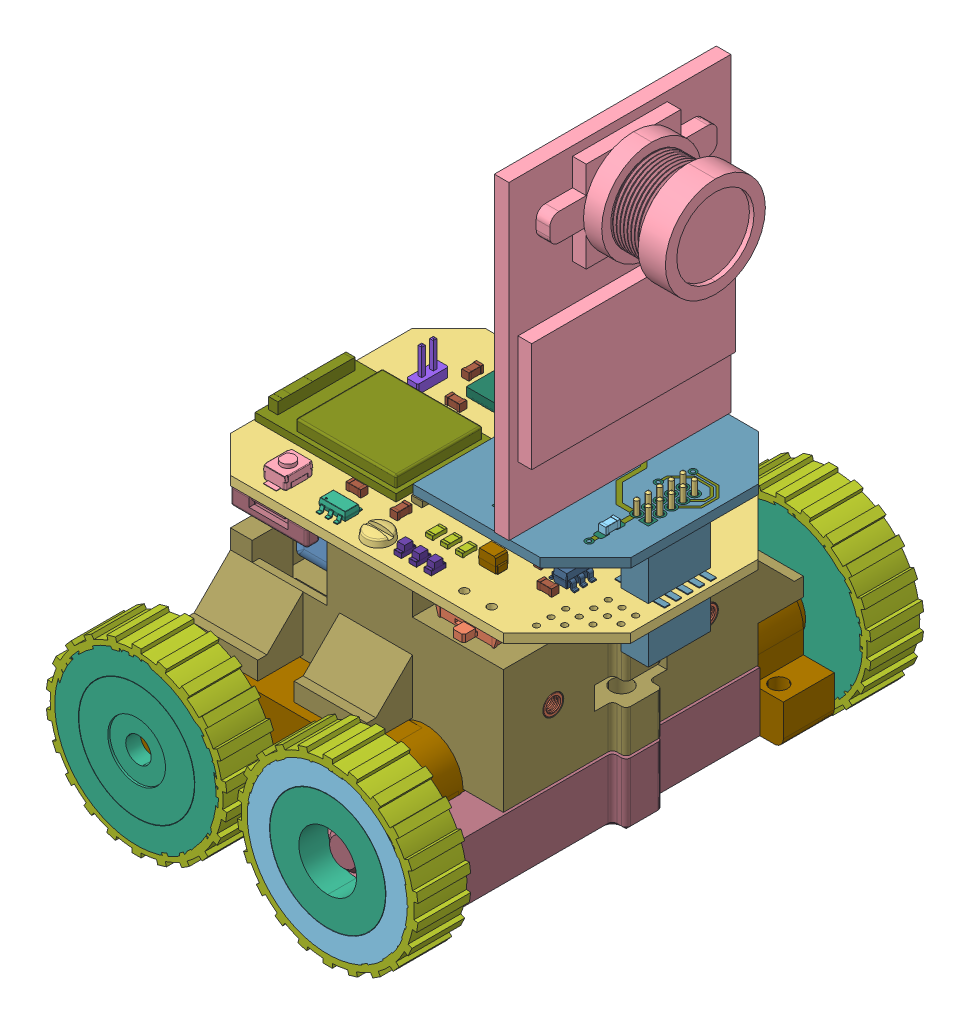
SolidWorks assembly AstroAnt_small_magnet, configuration Default. Lengths in mm.
Overall size (45.67 69.24 55.6).
158 component instances, 42 part files, 54 mates.
Components (placement in the parent):
- LiPo_360mAh-1: LiPo_360mAh [Default] at (6.8166 4.9998 44.2756) size (25 7 18)
- 92120A150_Brass Heat-Set Inserts for Plastic-1: 92120A150_Brass Heat-Set Inserts for Plastic [92120A150] at (19.9543 12.4998 45.7029) size (2.56 3.33 2.56)
- 92120A150_Brass Heat-Set Inserts for Plastic-2: 92120A150_Brass Heat-Set Inserts for Plastic [92120A150] at (4.9543 12.4998 33.9529) size (2.56 3.33 2.56)
- 92120A150_Brass Heat-Set Inserts for Plastic-3: 92120A150_Brass Heat-Set Inserts for Plastic [92120A150] at (4.9543 12.4998 57.4529) size (2.56 3.33 2.56)
- 91460A005_METRIC CHEESE HEAD SLOTTED MACHINE SCREW-8: 91460A005_METRIC CHEESE HEAD SLOTTED MACHINE SCREW [91460A005] at (4.9543 14.9998 57.4529) x (1 0 0) z (0 1 0) size (3 3 7.1)
- 91460A005_METRIC CHEESE HEAD SLOTTED MACHINE SCREW-9: 91460A005_METRIC CHEESE HEAD SLOTTED MACHINE SCREW [91460A005] at (4.9543 14.9998 33.9529) x (1 0 0) z (0 1 0) size (3 3 7.1)
- 91460A005_METRIC CHEESE HEAD SLOTTED MACHINE SCREW-10: 91460A005_METRIC CHEESE HEAD SLOTTED MACHINE SCREW [91460A005] at (19.9543 14.9998 45.7029) x (1 0 0) z (0 1 0) size (3 3 7.1)
- 92120A150_Brass Heat-Set Inserts for Plastic-4: 92120A150_Brass Heat-Set Inserts for Plastic [92120A150] at (4.9543 -0.6002 57.4529) x (-0.616962 0 -0.786993) z (0.786993 0 -0.616962) size (2.56 3.33 2.56)
- 92120A150_Brass Heat-Set Inserts for Plastic-5: 92120A150_Brass Heat-Set Inserts for Plastic [92120A150] at (4.9543 -0.6002 33.9529) x (-0.616962 0 -0.786993) z (0.786993 0 -0.616962) size (2.56 3.33 2.56)
- mainboard_v1.step-1: mainboard_v1.step [Default] at (-103.0457 13.9998 235.7029) x (0 0 -1) z (0 1 0) size (29.41 41 10.8)
  - B3U-1000P.step-1: B3U-1000P.step [Default] at (178.95 -97.38 1.05) x (1 0 0) z (0 -1 0) size (4 1.75 2.5)
    - COMPOUND.step-1: COMPOUND.step [Default] at origin size (4 1.75 2.5)
  - 20021321-00014C1LF.step-1: 20021321-00014C1LF.step [Default] at (190 -115.5 1.05) size (9.35 5.45 4.85)
    - COMPOUND-0.step-1: COMPOUND-0.step [Default] at origin size (9.35 5.45 4.85)
  - MP6513GJ-Z.step-1: MP6513GJ-Z.step [Default] at (201.21 -120 1.05) x (-1 0 0) z (0 0 1) size (2.8 2.9 1)
    - COMPOUND-1.step-1: COMPOUND-1.step [Default] at origin size (2.8 2.9 1)
  - MP6513GJ-Z.step-2: MP6513GJ-Z.step [Default] at (178.51 -103.46 1.05) size (2.8 2.9 1)
    - COMPOUND-1.step-1: COMPOUND-1.step [Default] at origin size (2.8 2.9 1)
  - R_0603_1608Metric.step-1: R_0603_1608Metric.step [Default] at (195.55 -104.38 -0.05) x (1 0 0) z (0 0 -1) size (1.6 0.8 0.45)
    - SOLID.step-1: SOLID.step [Default] at origin size (1.6 0.8 0.45)
  - R_0603_1608Metric.step-2: R_0603_1608Metric.step [Default] at (192.6 -99.86 -0.05) x (0 1 0) z (0 0 -1) size (1.6 0.8 0.45)
    - SOLID.step-1: SOLID.step [Default] at origin size (1.6 0.8 0.45)
  - PinHeader_2x01_P1.27mm_Vertical.step-1: PinHeader_2x01_P1.27mm_Vertical.step [Default] at (194.96 -96.07 1.05) size (3.4 1.27 6.3)
    - SOLID-2.step-1: SOLID-2.step [Default] at origin size (3.4 1.27 6.3)
  - TAJP106K010RNJ.step-1: TAJP106K010RNJ.step [Default] at (196.22 -98.14 -0.05) x (-1 0 0) z (0 0 -1) size (2.05 1.4 1.7)
    - COMPOUND-3.step-1: COMPOUND-3.step [Default] at origin size (2.05 1.4 1.7)
  - TAJP106K010RNJ.step-2: TAJP106K010RNJ.step [Default] at (181.68 -117.23 1.05) x (0 1 0) z (0 0 1) size (2.05 1.4 1.7)
    - COMPOUND-3.step-1: COMPOUND-3.step [Default] at origin size (2.05 1.4 1.7)
  - SOT-23-5.step-1: SOT-23-5.step [Default] at (195.38 -122.78 1.05) x (0 1 0) z (0 0 1) size (2.8 2.9 1.55)
    - SOLID-4.step-1: SOLID-4.step [Default] at origin size (2.8 2.9 1.55)
  - C_0603_1608Metric.step-1: C_0603_1608Metric.step [Default] at (192.91 -122.55 1.05) x (0 -1 0) z (0 0 1) size (1.6 0.8 0.8)
    - SOLID-5.step-1: SOLID-5.step [Default] at origin size (1.6 0.8 0.8)
  - C_0603_1608Metric.step-2: C_0603_1608Metric.step [Default] at (193.57 -119.76 1.05) size (1.6 0.8 0.8)
    - SOLID-5.step-1: SOLID-5.step [Default] at origin size (1.6 0.8 0.8)
  - ECS-.327-12.5-12-TR.step-1: ECS-.327-12.5-12-TR.step [Default] at (184.31 -107.18 1.05) size (2 1.2 0.7)
    - COMPOUND-6.step-1: COMPOUND-6.step [Default] at origin size (2 1.2 0.7)
  - C_0603_1608Metric.step-3: C_0603_1608Metric.step [Default] at (197.67 -113.69 1.05) size (1.6 0.8 0.8)
    - SOLID-5.step-1: SOLID-5.step [Default] at origin size (1.6 0.8 0.8)
  - C_0603_1608Metric.step-4: C_0603_1608Metric.step [Default] at (197.64 -107.18 1.05) size (1.6 0.8 0.8)
    - SOLID-5.step-1: SOLID-5.step [Default] at origin size (1.6 0.8 0.8)
  - C_0603_1608Metric.step-5: C_0603_1608Metric.step [Default] at (190.96 -108.09 1.05) x (0 1 0) z (0 0 1) size (1.6 0.8 0.8)
    - SOLID-5.step-1: SOLID-5.step [Default] at origin size (1.6 0.8 0.8)
  - 1734592-6.step-1: 1734592-6.step [Default] at (203.79 -118 -1.05) x (0 -1 0) z (1 0 0) size (8.43 2.05 5.11)
    - SOLID-7.step-1: SOLID-7.step [Default] at origin size (8.43 2.05 5.11)
  - 1734592-6.step-2: 1734592-6.step [Default] at (176.19 -98 -1.05) x (0 1 0) z (-1 0 0) size (8.43 2.05 5.11)
    - SOLID-7.step-1: SOLID-7.step [Default] at origin size (8.43 2.05 5.11)
  - 20021321-00010C4LF.step-1: 20021321-00010C4LF.step [Default] at (190 -127.85 -0.05) x (1 0 0) z (0 0 -1) size (6.81 5.45 4.85)
    - COMPOUND-8.step-1: COMPOUND-8.step [Default] at origin size (6.81 5.45 4.85)
  - 20021321-00010C4LF.step-2: 20021321-00010C4LF.step [Default] at (190 -127.85 1.05) size (6.81 5.45 4.85)
    - COMPOUND-8.step-1: COMPOUND-8.step [Default] at origin size (6.81 5.45 4.85)
  - C_0603_1608Metric.step-6: C_0603_1608Metric.step [Default] at (181.31 -102.6 1.05) x (0 -1 0) z (0 0 1) size (1.6 0.8 0.8)
    - SOLID-5.step-1: SOLID-5.step [Default] at origin size (1.6 0.8 0.8)
  - C_0603_1608Metric.step-7: C_0603_1608Metric.step [Default] at (198.25 -119.14 1.05) x (0 -1 0) z (0 0 1) size (1.6 0.8 0.8)
    - SOLID-5.step-1: SOLID-5.step [Default] at origin size (1.6 0.8 0.8)
  - MPU6050.step-1: MPU6050.step [Default] at (198.43 -101.5 1.05) x (0 1 0) z (1 0 0) size (4 0.95 4)
    - COMPOUND-9.step-1: COMPOUND-9.step [Default] at origin size (4 0.95 4)
  - C_0603_1608Metric.step-8: C_0603_1608Metric.step [Default] at (194.9 -99.89 1.05) x (0 -1 0) z (0 0 1) size (1.6 0.8 0.8)
    - SOLID-5.step-1: SOLID-5.step [Default] at origin size (1.6 0.8 0.8)
  - C_0603_1608Metric.step-9: C_0603_1608Metric.step [Default] at (201.98 -100.38 1.05) x (0 -1 0) z (0 0 1) size (1.6 0.8 0.8)
    - SOLID-5.step-1: SOLID-5.step [Default] at origin size (1.6 0.8 0.8)
  - C_0603_1608Metric.step-10: C_0603_1608Metric.step [Default] at (201.98 -103.78 1.05) x (0 1 0) z (0 0 1) size (1.6 0.8 0.8)
    - SOLID-5.step-1: SOLID-5.step [Default] at origin size (1.6 0.8 0.8)
  - C_0603_1608Metric.step-11: C_0603_1608Metric.step [Default] at (198.81 -97.82 1.05) size (1.6 0.8 0.8)
    - SOLID-5.step-1: SOLID-5.step [Default] at origin size (1.6 0.8 0.8)
  - SOT-23-5.step-2: SOT-23-5.step [Default] at (184.86 -122.77 1.05) x (0 1 0) z (0 0 1) size (2.8 2.9 1.55)
    - SOLID-4.step-1: SOLID-4.step [Default] at origin size (2.8 2.9 1.55)
  - SOT-23-5.step-3: SOT-23-5.step [Default] at (197.58 -110.46 1.05) x (0 1 0) z (0 0 1) size (2.8 2.9 1.55)
    - SOLID-4.step-1: SOLID-4.step [Default] at origin size (2.8 2.9 1.55)
  - MDBT50Q-1MV2.step-1: MDBT50Q-1MV2.step [Default] at (187.3136 -98.605 1.0754) x (-1 0 0) z (0 1 0) size (10.5 2.06 15.5)
    - SOLID-10.step-1: SOLID-10.step [Default] at origin size (10.5 2.06 15.5)
  - C_0603_1608Metric.step-12: C_0603_1608Metric.step [Default] at (189.44 -108.09 1.05) x (0 1 0) z (0 0 1) size (1.6 0.8 0.8)
    - SOLID-5.step-1: SOLID-5.step [Default] at origin size (1.6 0.8 0.8)
  - C_0603_1608Metric.step-13: C_0603_1608Metric.step [Default] at (181.57 -107.18 1.05) x (-1 0 0) z (0 0 1) size (1.6 0.8 0.8)
    - SOLID-5.step-1: SOLID-5.step [Default] at origin size (1.6 0.8 0.8)
  - C_0603_1608Metric.step-14: C_0603_1608Metric.step [Default] at (186.97 -107.18 1.05) size (1.6 0.8 0.8)
    - SOLID-5.step-1: SOLID-5.step [Default] at origin size (1.6 0.8 0.8)
  - C_0603_1608Metric.step-15: C_0603_1608Metric.step [Default] at (184.77 -119.75 1.05) x (-1 0 0) z (0 0 1) size (1.6 0.8 0.8)
    - SOLID-5.step-1: SOLID-5.step [Default] at origin size (1.6 0.8 0.8)
  - C_0603_1608Metric.step-16: C_0603_1608Metric.step [Default] at (182.37 -122.54 1.05) x (0 -1 0) z (0 0 1) size (1.6 0.8 0.8)
    - SOLID-5.step-1: SOLID-5.step [Default] at origin size (1.6 0.8 0.8)
  - LED_0603_1608Metric.step-1: LED_0603_1608Metric.step [Default] at (178.19 -111.01 1.05) size (1.6 0.8 1.1)
    - SOLID-11.step-1: SOLID-11.step [Default] at origin size (1.6 0.8 1.1)
  - LED_0603_1608Metric.step-2: LED_0603_1608Metric.step [Default] at (178.19 -112.66 1.05) size (1.6 0.8 1.1)
    - SOLID-11.step-1: SOLID-11.step [Default] at origin size (1.6 0.8 1.1)
  - LED_0603_1608Metric.step-3: LED_0603_1608Metric.step [Default] at (178.19 -114.31 1.05) size (1.6 0.8 1.1)
    - SOLID-11.step-1: SOLID-11.step [Default] at origin size (1.6 0.8 1.1)
  - LED_0603_1608Metric.step-4: LED_0603_1608Metric.step [Default] at (202.34 -112.21 1.05) x (0 1 0) z (0 0 1) size (1.6 0.8 1.1)
    - SOLID-11.step-1: SOLID-11.step [Default] at origin size (1.6 0.8 1.1)
  - 473460001.step-1: 473460001.step [Default] at (201.68 -99.72 -1.25) x (0 -1 0) z (1 0 0) size (7.98 2.94 5.43)
    - COMPOUND-12.step-1: COMPOUND-12.step [Default] at origin size (7.98 2.94 5.43)
  - L_0603_1608Metric.step-1: L_0603_1608Metric.step [Default] at (192.48 -108.09 1.05) x (0 1 0) z (0 0 1) size (1.6 0.8 0.8)
    - SOLID-13.step-1: SOLID-13.step [Default] at origin size (1.6 0.8 0.8)
  - R_0603_1608Metric.step-3: R_0603_1608Metric.step [Default] at (185.18 -111.31 1.05) x (-1 0 0) z (0 0 1) size (1.6 0.8 0.45)
    - SOLID.step-1: SOLID.step [Default] at origin size (1.6 0.8 0.45)
  - R_0603_1608Metric.step-4: R_0603_1608Metric.step [Default] at (185.18 -109.77 1.05) size (1.6 0.8 0.45)
    - SOLID.step-1: SOLID.step [Default] at origin size (1.6 0.8 0.45)
  - R_0603_1608Metric.step-5: R_0603_1608Metric.step [Default] at (181.62 -111.01 1.05) size (1.6 0.8 0.45)
    - SOLID.step-1: SOLID.step [Default] at origin size (1.6 0.8 0.45)
  - R_0603_1608Metric.step-6: R_0603_1608Metric.step [Default] at (181.62 -112.66 1.05) size (1.6 0.8 0.45)
    - SOLID.step-1: SOLID.step [Default] at origin size (1.6 0.8 0.45)
  - R_0603_1608Metric.step-7: R_0603_1608Metric.step [Default] at (181.62 -114.31 1.05) x (-1 0 0) z (0 0 1) size (1.6 0.8 0.45)
    - SOLID.step-1: SOLID.step [Default] at origin size (1.6 0.8 0.45)
  - R_0603_1608Metric.step-8: R_0603_1608Metric.step [Default] at (194.84 -108.1 1.05) x (0 1 0) z (0 0 1) size (1.6 0.8 0.45)
    - SOLID.step-1: SOLID.step [Default] at origin size (1.6 0.8 0.45)
  - R_0603_1608Metric.step-9: R_0603_1608Metric.step [Default] at (200.69 -112.2325 1.05) x (0 1 0) z (0 0 1) size (1.6 0.8 0.45)
    - SOLID.step-1: SOLID.step [Default] at origin size (1.6 0.8 0.45)
  - R_0603_1608Metric.step-10: R_0603_1608Metric.step [Default] at (196.22 -101.51 -0.05) x (-1 0 0) z (0 0 -1) size (1.6 0.8 0.45)
    - SOLID.step-1: SOLID.step [Default] at origin size (1.6 0.8 0.45)
  - R_0603_1608Metric.step-11: R_0603_1608Metric.step [Default] at (196.22 -99.9725 -0.05) x (-1 0 0) z (0 0 -1) size (1.6 0.8 0.45)
    - SOLID.step-1: SOLID.step [Default] at origin size (1.6 0.8 0.45)
  - SW_SPDT_PCM12.step-1: SW_SPDT_PCM12.step [Default] at (178.18 -119.37 -0.05) x (0 1 0) z (0 0 -1) size (7.7 5 2)
    - SOLID-14.step-1: SOLID-14.step [Default] at origin size (7.7 5 2)
  - COMPOUND-15.step-1: COMPOUND-15.step [Default] at origin size (28 41 1)
- ball_bearing_5x11x4mm-1: ball_bearing_5x11x4mm [Default] at (-65.9801 -4.7758 21.2029) x (0.999925 -0.012245 0) z (0 0 1) size (8 8 2.5)
- wheel_holder_non_motor-1: wheel_holder_non_motor [Default] at (-90.7699 -0.8362 17.9029) size (17.7 17.7 5.8)
- wheel_holder_non_motor-2: wheel_holder_non_motor [Default] at (1.3792 -86.6559 73.5029) x (0.185441 0.982655 0) z (0 0 -1) size (17.7 17.7 5.8)
- ball_bearing_5x11x4mm-2: ball_bearing_5x11x4mm [Default] at (-9.788 -57.5376 70.2029) x (0.373101 0.927791 0) z (0 0 -1) size (8 8 2.5)
- wheel_motor-1: wheel_motor [Default] at (44.5289 -0.8963 17.9029) size (18 18 5.8)
- wheel_motor-2: wheel_motor [Default] at (-4.9746 26.526 73.5029) x (-0.038296 0.999266 0) z (0 0 -1) size (18 18 5.8)
- tire-1: tire [Default] at (58.6593 -4.042 17.9029) size (19.84 19.9 5.8)
- tire-2: tire [Default] at (37.6493 -4.042 17.9029) size (19.84 19.9 5.8)
- tire-3: tire [Default] at (58.6593 -4.042 67.7029) size (19.84 19.9 5.8)
- tire-4: tire [Default] at (37.6493 -4.042 67.7029) size (19.84 19.9 5.8)
- PA2-50_with_gearbox-3: PA2-50_with_gearbox [Default] at (45.51 -3.6027 60.1029) x (-1 0 0) z (0 0 1) size (30.92 12.52 38.5)
  - PA2-50-1: PA2-50 [Default] at (26.117 -19.7771 -19.1) x (0 0 1) z (0.954024 0.299729 0) size (29.1 8 8)
  - gearbox-1: gearbox [Default] at origin size (29.9 11.5 13.6)
- PA2-50_with_gearbox-4: PA2-50_with_gearbox [Default] at (-35.6268 -3.6027 31.3029) x (1 0 0) z (0 0 -1) size (30.92 12.52 38.5)
  - PA2-50-1: PA2-50 [Default] at (26.117 -19.7771 -19.1) x (0 0 1) z (0.954024 0.299729 0) size (29.1 8 8)
  - gearbox-1: gearbox [Default] at origin size (29.9 11.5 13.6)
- TPiS_1084-1: TPiS_1084 [Default] at (-17.7438 -7.4002 31.4743) size (9.3 10.3 10.11)
- IR_TEMP_module-1: IR_TEMP_module [Default] at (15.0895 3.8498 50.7532) x (0 0 -1) z (0 1 0) size (10 20 1.85)
- robobody-1: robobody [Default] at (-9.0457 6.9406 -0.9986) size (31.5 16.1 38)
- 92120A150_Brass Heat-Set Inserts for Plastic-6: 92120A150_Brass Heat-Set Inserts for Plastic [92120A150] at (19.9543 -0.6002 45.7029) x (-0.616962 0 -0.786993) z (0.786993 0 -0.616962) size (2.56 3.33 2.56)
- motor_holder_2-1: motor_holder_2 [Default] at (52.4112 -9.4002 -5.2676) size (31.5 8.8 52.2)
- 92120A150_Brass Heat-Set Inserts for Plastic-7: 92120A150_Brass Heat-Set Inserts for Plastic [92120A150] at (19.4543 5.3998 54.2029) x (0 1 0) z (0 0 1) size (2.56 3.33 2.56)
- 92120A150_Brass Heat-Set Inserts for Plastic-8: 92120A150_Brass Heat-Set Inserts for Plastic [92120A150] at (19.4543 5.3998 37.2029) x (0 1 0) z (0 0 1) size (2.56 3.33 2.56)
- Camera1-Camera.step-1: Camera1-Camera.step [Default] at (-70.9957 22.1998 197.7029) x (0 0 -1) z (0 1 0) size (24.4 21.18 39.4)
  - Board_Geoms_150e.step-1: Board_Geoms_150e.step [Default] at origin size (24 19 1.05)
    - Pcb_150e.step-1: Pcb_150e.step [Default] at origin size (24 19 1)
    - topPads_150e.step-1: topPads_150e.step [Default] at (0 0 0.02) size (19.49 14.67 0.01)
    - topTracks_150e.step-1: topTracks_150e.step [Default] at (0 0 0.01) size (12.72 10.5 0.01)
    - botPads_150e.step-1: botPads_150e.step [Default] at (0 0 -1.02) size (19.49 14.67 0.01)
    - botTracks_150e.step-1: botTracks_150e.step [Default] at (0 0 -1.01) size (18.04 10.2 0.01)
    - botZones_150e.step-1: botZones_150e.step [Default] at (0 0 -1.01) size (23.45 18.45 0.01)
  - Step_Models_150e.step-1: Step_Models_150e.step [Default] at origin size (24.4 19.37 39.4)
    - Top_150e.step-1: Top_150e.step [Default] at origin size (24.4 19.37 39.4)
      - J2_ASSEMBLY_61432F3D.step-1: J2_ASSEMBLY_61432F3D.step [Default] at (149.47 -82.87 -1) x (1 0 0) z (0 0 -1) size (6.35 3.4 6.9)
        - Body.step-1: Body.step [Default] at origin size (6.35 3.4 1.3)
        - LeadsArray.step-1: LeadsArray.step [Default] at origin size (5.58 1.77 6.9)
      - J2_ASSEMBLY_61432F3D.step-2: J2_ASSEMBLY_61432F3D.step [Default] at (149.46 -95.165 -1) x (1 0 0) z (0 0 -1) size (6.35 3.4 6.9)
        - Body.step-1: Body.step [Default] at origin size (6.35 3.4 1.3)
        - LeadsArray.step-1: LeadsArray.step [Default] at origin size (5.58 1.77 6.9)
      - U1_Arducam_OV2640_61432450.step-1: U1_Arducam_OV2640_61432450.step [Default] at (150.125 -88.26 0) x (-1 0 0) z (0 0 1) size (24.4 13.6 34.1)
      - C1_C_0603_1608Metric_61432400.step-1: C1_C_0603_1608Metric_61432400.step [Default] at (146.47 -95.15 0) x (-1 0 0) z (0 0 1) size (1.6 0.8 0.8)
- R842-1: R842 [Default] at (-5.5634 -2.6002 71.9154) x (1 0 0) z (0 -1 0) size (12.7 3.17 12.7)
- R842-2: R842 [Default] at (15.4466 -2.6002 71.9154) x (1 0 0) z (0 -1 0) size (12.7 3.17 12.7)
- R842-3: R842 [Default] at (-5.5634 -2.6002 19.4904) x (1 0 0) z (0 -1 0) size (12.7 3.17 12.7)
- R842-4: R842 [Default] at (15.4466 -2.6002 19.4904) x (1 0 0) z (0 -1 0) size (12.7 3.17 12.7)
Mates (geometry in assembly coordinates):
- Concentric63: concentric anti-aligned: cylinder of ball_bearing_5x11x4mm-1 through (-5.5634 -2.6002 23.7029) axis (0 0 -1) radius 4; cylinder of wheel_holder_non_motor-1 through (-5.5634 -2.6002 17.9029) axis (0 0 1) radius 4
- Coincident105: coincident aligned: plane of ball_bearing_5x11x4mm-1 through (-5.5634 -2.6002 23.7029) normal (0 0 1); plane of wheel_holder_non_motor-1 through (-5.5634 -2.6002 23.7029) normal (0 0 1)
- Coincident107: coincident aligned: plane of wheel_holder_non_motor-2 through (15.4466 -2.6002 67.7029) normal (0 0 -1); plane of ball_bearing_5x11x4mm-2 through (15.4466 -2.6002 67.7029) normal (0 0 -1)
- Concentric83: concentric anti-aligned: cylinder of wheel_motor-1 through (15.4466 -2.6002 23.7029) axis (0 0 -1) radius 9; cylinder of tire-1 through (15.4466 -2.6002 17.9029) axis (0 0 1) radius 8.75
- Coincident123: coincident aligned: plane of wheel_motor-1 through (15.4466 -2.6002 17.9029) normal (0 0 -1); plane of tire-1 through (15.4466 -2.6002 17.9029) normal (0 0 -1)
- Concentric84: concentric anti-aligned: cylinder of wheel_holder_non_motor-1 through (-5.5634 -2.6002 23.7029) axis (0 0 -1) radius 8.85; cylinder of tire-2 through (-5.5634 -2.6002 17.9029) axis (0 0 1) radius 8.75
- Coincident124: coincident aligned: plane of wheel_holder_non_motor-1 through (-5.5634 -2.6002 17.9029) normal (0 0 -1); plane of tire-2 through (-5.5634 -2.6002 17.9029) normal (0 0 -1)
- Coincident125: coincident aligned: plane of wheel_motor-2 through (-5.5634 -2.6002 73.5029) normal (0 0 1); plane of tire-4 through (-5.5634 -2.6002 73.5029) normal (0 0 1)
- Concentric85: concentric aligned: cylinder of wheel_motor-2 through (-5.5634 -2.6002 67.7029) axis (0 0 1) radius 9; cylinder of tire-4 through (-5.5634 -2.6002 67.7029) axis (0 0 1) radius 8.75
- Coincident126: coincident aligned: plane of wheel_holder_non_motor-2 through (15.4466 -2.6002 73.5029) normal (0 0 1); plane of tire-3 through (15.4466 -2.6002 73.5029) normal (0 0 1)
- Concentric86: concentric aligned: cylinder of wheel_holder_non_motor-2 through (15.4466 -2.6002 67.7029) axis (0 0 1) radius 8.85; cylinder of tire-3 through (15.4466 -2.6002 67.7029) axis (0 0 1) radius 8.75
- Concentric100: concentric anti-aligned: cylinder of wheel_holder_non_motor-2 through (15.4466 -2.6002 73.5029) axis (0 0 -1) radius 4; cylinder of ball_bearing_5x11x4mm-2 through (15.4466 -2.6002 66.2029) axis (0 0 1) radius 2
- Coincident138: coincident aligned: plane of wheel_holder_non_motor-2 through (15.4466 -2.6002 67.7029) normal (0 0 -1); plane of ball_bearing_5x11x4mm-2 through (15.4466 -2.6002 67.7029) normal (0 0 -1)
- Concentric110: concentric anti-aligned: cylinder of wheel_motor-2 through (-5.5634 -2.6002 67.7029) axis (0 0 1) radius 1.4; cylinder of PA2-50_with_gearbox-3/gearbox-1 through (-5.5634 -2.6002 71.7029) axis (0 0 -1) radius 1.45
- Concentric111: concentric aligned: cylinder of tire-1 through (15.4466 -2.6002 23.7029) axis (0 0 -1) radius 9.5; cylinder of tire-3 through (15.4466 -2.6002 73.5029) axis (0 0 -1) radius 9.5
- Concentric112: concentric aligned: cylinder of tire-2 through (-5.5634 -2.6002 23.7029) axis (0 0 -1) radius 9.5; cylinder of tire-4 through (-5.5634 -2.6002 73.5029) axis (0 0 -1) radius 9.5
- Coincident144: coincident aligned: plane of PA2-50_with_gearbox-3/gearbox-1 through (16.4366 -9.1002 65.7029) normal (0 -1 0); plane of PA2-50_with_gearbox-4/gearbox-1 through (-6.5534 -9.1002 25.7029) normal (0 -1 0)
- Coincident145: coincident aligned: plane of wheel_holder_non_motor-1 through (-5.5634 -2.6002 17.9029) normal (0 0 -1); plane of wheel_motor-1 through (15.4466 -2.6002 17.9029) normal (0 0 -1)
- Coincident146: coincident aligned: plane of wheel_holder_non_motor-2 through (15.4466 -2.6002 73.5029) normal (0 0 1); plane of wheel_motor-2 through (-5.5634 -2.6002 73.5029) normal (0 0 1)
- Concentric118: concentric anti-aligned: cylinder of TPiS_1084-1 through (2.2416 -0.7002 46.8203) axis (0 -1 0) radius 0.225; cylinder of IR_TEMP_module-1 through (2.2414 3.8498 46.8208) axis (0 1 0) radius 0.3
- Concentric119: concentric anti-aligned: cylinder of TPiS_1084-1 through (3.8219 -0.7002 43.0052) axis (0 -1 0) radius 0.225; cylinder of IR_TEMP_module-1 through (3.8219 3.8498 43.0052) axis (0 1 0) radius 0.3
- Coincident153: coincident aligned: plane of mainboard_v1.step-1/COMPOUND-15.step-1 through (20.9543 13.9998 59.7029) normal (0 0 1); plane of robobody-1 through (20.9543 13.9998 59.7029) normal (0 0 1)
- Coincident154: coincident: line of mainboard_v1.step-1/COMPOUND-15.step-1 through (-9.0457 13.9998 59.7029) axis (0 1 0); plane of robobody-1 through (-9.0457 6.9406 -0.9986) normal (-1 0 0)
- Parallel1: parallel: line of IR_TEMP_module-1 through (15.0895 3.8498 50.7532) axis (-1 0 0); plane of robobody-1 through (-8.0457 3.9998 55.2029) normal (0 0 -1)
- Concentric121: concentric aligned: cylinder of 92120A150_Brass Heat-Set Inserts for Plastic-4 through (4.9543 0.8998 57.4529) axis (0 1 0) radius 1.075; cylinder of robobody-1 through (4.9543 -2.1591 57.4529) axis (0 1 0) radius 1.15
- Concentric122: concentric aligned: cylinder of 92120A150_Brass Heat-Set Inserts for Plastic-5 through (4.9543 0.8998 33.9529) axis (0 1 0) radius 1.075; cylinder of robobody-1 through (4.9543 -2.1591 33.9529) axis (0 1 0) radius 1.15
- Concentric123: concentric aligned: cylinder of robobody-1 through (19.9543 -2.1591 45.7029) axis (0 1 0) radius 1.15; cylinder of 92120A150_Brass Heat-Set Inserts for Plastic-6 through (19.9543 0.8998 45.7029) axis (0 1 0) radius 1.075
- Coincident164: coincident anti-aligned: plane of PA2-50_with_gearbox-4/gearbox-1 through (12.2966 -5.4002 30.3029) normal (0 -1 0); plane of motor_holder_2-1 through (-9.0457 -5.4002 31.5029) normal (0 1 0)
- Coincident167: coincident aligned: plane of robobody-1 through (20.9543 6.9406 -0.9986) normal (1 0 0); plane of motor_holder_2-1 through (20.9543 -2.4002 61.1029) normal (1 0 0)
- Coincident168: coincident anti-aligned: plane of TPiS_1084-1 through (4.9393 -7.4002 45.7029) normal (0 -1 0); plane of motor_holder_2-1 through (4.9393 -7.4002 45.7029) normal (0 1 0)
- Coincident169: coincident anti-aligned: plane of TPiS_1084-1 through (4.9393 -7.4002 45.7029) normal (0 -1 0); plane of motor_holder_2-1 through (4.9393 -7.4002 45.7029) normal (0 1 0)
- Coincident170: coincident anti-aligned: plane of TPiS_1084-1 through (4.9393 -7.4002 45.7029) normal (0 -1 0); plane of motor_holder_2-1 through (4.9393 -7.4002 45.7029) normal (0 1 0)
- Concentric124: concentric anti-aligned: cylinder of PA2-50_with_gearbox-3/PA2-50-1 through (12.4366 -2.1002 57.2029) axis (0 0 -1) radius 4; cylinder of robobody-1 through (12.4366 -2.1002 32.5029) axis (0 0 1) radius 4.1
- Concentric125: concentric anti-aligned: cylinder of PA2-50_with_gearbox-4/PA2-50-1 through (-2.5534 -2.1002 34.2029) axis (0 0 1) radius 4; cylinder of robobody-1 through (-2.5534 -2.1002 58.9029) axis (0 0 -1) radius 4.1
- Coincident174: coincident anti-aligned: plane of PA2-50_with_gearbox-4/gearbox-1 through (-2.5534 -2.1002 31.7029) normal (0 0 1); plane of robobody-1 through (20.9543 13.9998 31.7029) normal (0 0 -1)
- Coincident175: coincident anti-aligned: plane of PA2-50_with_gearbox-3/gearbox-1 through (12.4366 -2.1002 59.7029) normal (0 0 -1); plane of robobody-1 through (20.9543 13.9998 59.7029) normal (0 0 1)
- Coincident176: coincident anti-aligned: plane of mainboard_v1.step-1/COMPOUND-15.step-1 through (6.7692 13.9998 45.7029) normal (0 -1 0); plane of robobody-1 through (20.9543 13.9998 59.7029) normal (0 1 0)
- Concentric126: concentric anti-aligned: cylinder of robobody-1 through (14.5016 5.3998 54.2029) axis (1 0 0) radius 1.15; cylinder of 92120A150_Brass Heat-Set Inserts for Plastic-7 through (17.9543 5.3998 54.2029) axis (-1 0 0) radius 1.075
- Concentric127: concentric anti-aligned: cylinder of robobody-1 through (14.5016 5.3998 37.2029) axis (1 0 0) radius 1.15; cylinder of 92120A150_Brass Heat-Set Inserts for Plastic-8 through (17.9543 5.3998 37.2029) axis (-1 0 0) radius 1.075
- Coincident177: coincident aligned: plane of robobody-1 through (20.9543 6.9406 -0.9986) normal (1 0 0); plane of 92120A150_Brass Heat-Set Inserts for Plastic-8 through (20.9543 4.5998 37.2029) normal (1 0 0)
- Coincident178: coincident aligned: plane of robobody-1 through (20.9543 6.9406 -0.9986) normal (1 0 0); plane of 92120A150_Brass Heat-Set Inserts for Plastic-7 through (20.9543 4.5998 54.2029) normal (1 0 0)
- Distance1: distance = 2 mm anti-aligned: plane of wheel_motor-2 through (-5.5634 -2.6002 67.7029) normal (0 0 -1); plane of PA2-50_with_gearbox-3/gearbox-1 through (45.51 -3.6027 65.7029) normal (0 0 1)
- Distance2: distance = 2 mm anti-aligned: plane of wheel_motor-1 through (15.4466 -2.6002 23.7029) normal (0 0 1); plane of PA2-50_with_gearbox-4/gearbox-1 through (-35.6268 -3.6027 25.7029) normal (0 0 -1)
- Coincident182: coincident anti-aligned: plane of mainboard_v1.step-1/20021321-00010C4LF.step-2/COMPOUND-8.step-1 through (24.8043 19.8998 45.7029) normal (0 1 0); plane of Camera1-Camera.step-1/Step_Models_150e.step-1/Top_150e.step-1/J2_ASSEMBLY_61432F3D.step-2/Body.step-1 through (23.1043 19.8998 48.8779) normal (0 -1 0)
- Distance3: distance = 0.23 mm aligned: plane of Camera1-Camera.step-1/Step_Models_150e.step-1/Top_150e.step-1/J2_ASSEMBLY_61432F3D.step-2/Body.step-1 through (23.1043 21.1998 42.5279) normal (0 0 -1); plane of mainboard_v1.step-1/20021321-00010C4LF.step-2/COMPOUND-8.step-1 through (23.3043 15.1498 42.2979) normal (0 0 -1)
- Distance4: distance = 0.2 mm aligned: plane of Camera1-Camera.step-1/Step_Models_150e.step-1/Top_150e.step-1/J2_ASSEMBLY_61432F3D.step-2/Body.step-1 through (23.1043 21.1998 48.8779) normal (-1 0 0); plane of mainboard_v1.step-1/20021321-00010C4LF.step-2/COMPOUND-8.step-1 through (23.3043 15.1498 49.1079) normal (-1 0 0)
- Concentric128: concentric anti-aligned: cylinder of wheel_motor-2 through (-5.5634 -2.6002 70.3029) axis (0 0 1) radius 6.4; cylinder of R842-1 through (-5.5634 -2.6002 73.5029) axis (0 0 -1) radius 3.175
- Concentric129: concentric anti-aligned: cylinder of wheel_holder_non_motor-2 through (15.4466 -2.6002 70.3029) axis (0 0 1) radius 6.4; cylinder of R842-2 through (15.4466 -2.6002 73.5029) axis (0 0 -1) radius 3.175
- Coincident183: coincident aligned: plane of wheel_holder_non_motor-2 through (15.4466 -2.6002 73.5029) normal (0 0 1); plane of R842-2 through (15.4466 -2.6002 73.5029) normal (0 0 1)
- Coincident184: coincident aligned: plane of wheel_motor-2 through (-5.5634 -2.6002 73.5029) normal (0 0 1); plane of R842-1 through (-5.5634 -2.6002 73.5029) normal (0 0 1)
- Concentric130: concentric aligned: cylinder of wheel_motor-1 through (15.4466 -2.6002 21.1029) axis (0 0 -1) radius 3.15; cylinder of R842-4 through (15.4466 -2.6002 21.0779) axis (0 0 -1) radius 3.175
- Coincident185: coincident aligned: plane of wheel_motor-1 through (15.4466 -2.6002 17.9029) normal (0 0 -1); plane of R842-4 through (15.4466 -2.6002 17.9029) normal (0 0 -1)
- Concentric131: concentric aligned: cylinder of wheel_holder_non_motor-1 through (-5.5634 -2.6002 21.1029) axis (0 0 -1) radius 6.4; cylinder of R842-3 through (-5.5634 -2.6002 21.0779) axis (0 0 -1) radius 6.35
- Coincident186: coincident aligned: plane of wheel_holder_non_motor-1 through (-5.5634 -2.6002 17.9029) normal (0 0 -1); plane of R842-3 through (-5.5634 -2.6002 17.9029) normal (0 0 -1)
